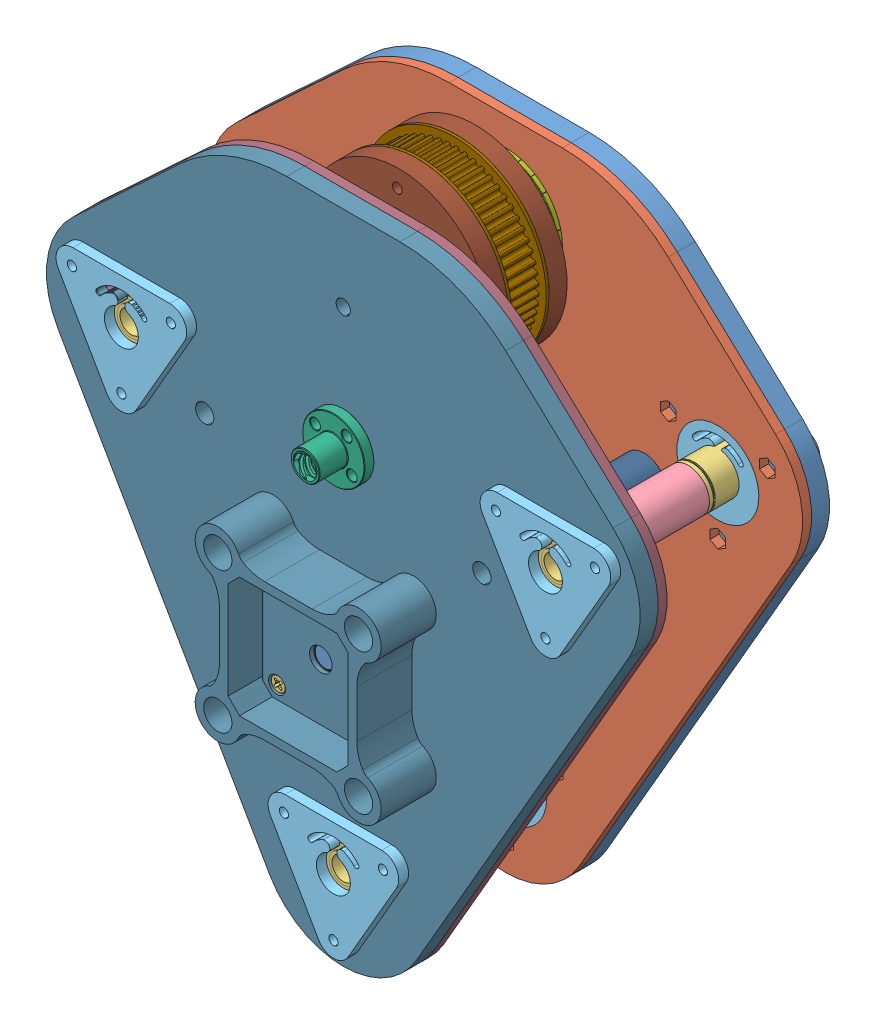
SolidWorks assembly assemblage_chariot, configuration Défaut. Lengths in mm.
Overall size (210 235.26 100).
51 component instances, 32 part files, 108 mates.
Components (placement in the parent):
- chariot_1_4_axe_z-1: chariot_1_4_axe_z [Défaut] at (104.2914 -77.7812 228.825) size (210 232 13.03)
- chariot_1_8_axe_z-1: chariot_1_8_axe_z [Défaut] at (104.2914 -77.7812 235.175) size (210 232 13.03)
- LM8UU-1: LM8UU [Default] at (179.2914 22.2188 238.825) x (-0.119175 0.992873 0) z (0 0 1) size (15 15 20)
- LM8UU-2: LM8UU [Default] at (104.2914 -107.7812 285.825) x (0.999936 0.011352 0) z (0 0 1) size (15 15 20)
- LM8UU-3: LM8UU [Default] at (29.2914 22.2188 285.825) x (0.609724 0.792614 0) z (0 0 1) size (15 15 20)
- LM8UU-4: LM8UU [Default] at (29.2914 22.2188 238.825) x (0.999283 -0.037866 0) z (0 0 1) size (15 15 20)
- LM8UU-5: LM8UU [Default] at (179.2914 22.2188 285.825) size (15 15 20)
- LM8UU-6: LM8UU [Default] at (104.2914 -107.7812 238.825) size (15 15 20)
- spacer_bearing_chariot-1: spacer_bearing_chariot [Défaut] at (104.2914 -107.7812 248.825) x (0.653682 -0.75677 0) z (0 0 1) size (15 15 27)
- spacer_bearing_chariot-2: spacer_bearing_chariot [Défaut] at (179.2914 22.2188 248.825) x (0.959506 -0.281688 0) z (0 0 1) size (15 15 27)
- spacer_bearing_chariot-3: spacer_bearing_chariot [Défaut] at (29.2914 22.2188 248.825) x (0.998603 0.052836 0) z (0 0 1) size (15 15 27)
- ancrage_bearing_lineaire-1: ancrage_bearing_lineaire [Défaut] at (179.2914 22.2188 299.325) x (-1 0 0) z (0 0 -1) size (46.22 41.63 13.03)
- ancrage_bearing_lineaire-2: ancrage_bearing_lineaire [Défaut] at (104.2914 -107.7812 299.325) x (-1 -0.000641 0) z (0 0 -1) size (46.22 41.63 13.03)
- ancrage_bearing_lineaire-3: ancrage_bearing_lineaire [Défaut] at (179.2914 22.2188 225.325) size (46.22 41.63 13.03)
- ancrage_bearing_lineaire-4: ancrage_bearing_lineaire [Défaut] at (104.2914 -107.7812 225.325) x (1 0.000641 0) z (0 0 1) size (46.22 41.63 13.03)
- ancrage_bearing_lineaire-5: ancrage_bearing_lineaire [Défaut] at (29.2914 22.2188 299.325) x (-1 -0.000641 0) z (0 0 -1) size (46.22 41.63 13.03)
- ancrage_bearing_lineaire-6: ancrage_bearing_lineaire [Défaut] at (29.2914 22.2188 225.325) size (46.22 41.63 13.03)
- Lead screw Nut tr8x8-4.step-1: Lead screw Nut tr8x8-4.step [Défaut] at (104.2914 22.2188 228.825) x (-0.445347 -0.895358 0) z (0 0 1) size (22 22 15)
- Lead screw Nut tr8x8-4.step-2: Lead screw Nut tr8x8-4.step [Défaut] at (104.2914 22.2188 295.825) x (0.811634 -0.584167 0) z (0 0 -1) size (22 22 15)
- 7806K755_Thrust Ball Bearing-1: 7806K755_Thrust Ball Bearing [7806K755] at (104.2914 64.2188 242.175) x (1 0 0) z (0 -1 0) size (40 14 40)
- 7806K755_Thrust Ball Bearing-2: 7806K755_Thrust Ball Bearing [7806K755] at (104.2914 64.2188 283.0983) x (-0.376178 0.926547 0) z (-0.926547 -0.376178 0) size (40 14 40)
- ThrustBallBearingUpper-1: ThrustBallBearingUpper [7806K755] at (104.2914 64.2188 242.1746) x (0.97097 0.239202 0) z (-0.239202 0.97097 0) size (40 14 40)
- ThrustBallBearingUpper-2: ThrustBallBearingUpper [7806K755] at (104.2914 64.2188 283.0986) x (0.933029 0.359801 0) z (0.359801 -0.933029 0) size (40 14 40)
- poulie_dente_modif-1: poulie_dente_modif [Výchozí] at (104.2914 64.2188 262.6366) x (0.023795 -0.999717 0) z (-0.999717 -0.023795 0) size (65 14.22 65)
- colonne_chariot-1: colonne_chariot [Défaut] at (153.3107 7.2188 238.35) size (16 16 48.51)
- colonne_chariot-2: colonne_chariot [Défaut] at (55.2722 7.2188 238.35) size (16 16 48.51)
- colonne_chariot-3: colonne_chariot [Défaut] at (104.2914 -79.7812 238.35) size (16 16 48.51)
- appuie_1_4_poulie-1: appuie_1_4_poulie [Default] at (104.2914 64.2188 255.5246) x (0.023795 -0.999717 0) z (0.999717 0.023795 0) size (65 6.35 65)
- appuie_1_4_poulie-2: appuie_1_4_poulie [Default] at (104.2914 64.2188 276.0986) x (-0.999717 -0.023795 0) z (0.023795 -0.999717 0) size (65 6.35 65)
- NEMA17 x 33.step-1: NEMA17 x 33.step [Défaut] at (104.2914 -39.7812 270.7486) x (1 0 0) z (0 -1 0) size (42 57 60)
  - Copper-2of4.step-1: Copper-2of4.step [Défaut] at (0 28 0) x (0 1 0) z (0 0 1) size (2.77 3.05 24)
  - Frontplate.step-1: Frontplate.step [Défaut] at (0 10.5 0) size (42 12.5 42)
  - Backplate.step-1: Backplate.step [Défaut] at (0 33 0) size (42 10.5 42)
  - Connenctor.step-1: Connenctor.step [Défaut] at (0 24.5 22) size (7 7 7)
  - Housing.step-1: Housing.step [Défaut] at (0 7.5 0) size (42 17 42)
  - Bearing dummy.step-1: Bearing dummy.step [Défaut] at (0 4 0) size (22 7 22)
  - Bearing dummy 01.step-1: Bearing dummy 01.step [Défaut] at (0 28 0) size (22 7 22)
  - Core.step-1: Core.step [Défaut] at origin size (30 55.5 30)
  - M3x25-Screw.step-1: M3x25-Screw.step [Défaut] at (15.5 30.6 15.5) x (1 0 0) z (0 1 0) size (5.5 5.5 27)
  - M3x25-Screw004.step-1: M3x25-Screw004.step [Défaut] at (-15.5 30.6 15.5) x (1 0 0) z (0 1 0) size (5.5 5.5 27)
  - M3x25-Screw005.step-1: M3x25-Screw005.step [Défaut] at (-15.5 30.6 -15.5) x (1 0 0) z (0 1 0) size (5.5 5.5 27)
  - M3x25-Screw006.step-1: M3x25-Screw006.step [Défaut] at (15.5 30.6 -15.5) x (1 0 0) z (0 1 0) size (5.5 5.5 27)
  - Cable-1of4.step-1: Cable-1of4.step [Défaut] at (0 28 0) size (3.44 3.69 21)
  - Copper-1of4.step-1: Copper-1of4.step [Défaut] at (0 28 0) size (2.77 3.05 24)
  - Cable-2of4.step-1: Cable-2of4.step [Défaut] at (0 28 0) x (0 1 0) z (0 0 1) size (3.44 3.69 21)
  - Copper-4of4.step-1: Copper-4of4.step [Défaut] at (0 28 0) x (0 -1 0) z (0 0 1) size (2.77 3.05 24)
  - Cable-3of4.step-1: Cable-3of4.step [Défaut] at (0 28 0) x (-1 0 0) z (0 0 1) size (3.44 3.69 21)
  - Copper-3of4.step-1: Copper-3of4.step [Défaut] at (0 28 0) x (-1 0 0) z (0 0 1) size (2.77 3.05 24)
  - Cable-4of4.step-1: Cable-4of4.step [Défaut] at (0 28 0) x (0 -1 0) z (0 0 1) size (3.44 3.69 21)
- chariot_1_8_axe_z_sans_trou_haut-2: chariot_1_8_axe_z_sans_trou_haut [Défaut] at (104.2914 -77.7812 286.3) size (210 232 13.03)
- chariot_1_4_axe_z_sans_trou_haut-2: chariot_1_4_axe_z_sans_trou_haut [Défaut] at (104.2914 -77.7812 289.475) size (210 232 29.35)
Mates (geometry in assembly coordinates):
- Coïncidente1: coincident anti-aligned: plane of chariot_1_4_axe_z-1 through (29.2914 22.2188 235.175) normal (0 0 1); plane of chariot_1_8_axe_z-1 through (29.2914 22.2188 235.175) normal (0 0 -1)
- Coaxiale1: concentric aligned: cylinder of chariot_1_4_axe_z-1 through (104.2914 22.2188 228.825) axis (0 0 1) radius 5.1; cylinder of chariot_1_8_axe_z-1 through (104.2914 22.2188 235.175) axis (0 0 1) radius 5.1
- Coaxiale2: concentric aligned: cylinder of chariot_1_4_axe_z-1 through (179.2914 22.2188 228.825) axis (0 0 1) radius 14.5; cylinder of chariot_1_8_axe_z-1 through (179.2914 22.2188 235.175) axis (0 0 1) radius 14.5
- Coïncidente2: coincident anti-aligned: plane of chariot_1_4_axe_z-2 through (29.2914 22.2188 290.007) normal (0 0 -1); plane of chariot_1_8_axe_z-2 through (29.2914 22.2188 290.007) normal (0 0 1)
- Coaxiale3: concentric aligned: cylinder of chariot_1_4_axe_z-2 through (179.2914 22.2188 290.007) axis (0 0 1) radius 14.5; cylinder of chariot_1_8_axe_z-2 through (179.2914 22.2188 286.832) axis (0 0 1) radius 8
- Coaxiale4: concentric aligned: cylinder of chariot_1_4_axe_z-2 through (104.2914 22.2188 290.007) axis (0 0 1) radius 5.1; cylinder of chariot_1_8_axe_z-2 through (104.2914 22.2188 286.832) axis (0 0 1) radius 5.1
- Coaxiale5: concentric aligned: cylinder of chariot_1_8_axe_z-1 through (29.2914 22.2188 235.175) axis (0 0 1) radius 14.5; cylinder of chariot_1_8_axe_z-2 through (29.2914 22.2188 286.832) axis (0 0 1) radius 8
- Coaxiale6: concentric aligned: cylinder of chariot_1_8_axe_z-1 through (179.2914 22.2188 235.175) axis (0 0 1) radius 14.5; cylinder of chariot_1_8_axe_z-2 through (179.2914 22.2188 286.832) axis (0 0 1) radius 8
- Coaxiale7: concentric anti-aligned: cylinder of chariot_1_8_axe_z-1 through (179.2914 22.2188 235.175) axis (0 0 1) radius 14.5; cylinder of LM8UU-1 through (179.2914 22.2188 248.825) axis (0 0 -1) radius 7.5
- Coaxiale8: concentric anti-aligned: cylinder of chariot_1_4_axe_z-1 through (104.2914 -107.7812 228.825) axis (0 0 1) radius 14.5; cylinder of LM8UU-6 through (104.2914 -107.7812 248.825) axis (0 0 -1) radius 7.5
- Coaxiale9: concentric anti-aligned: cylinder of chariot_1_4_axe_z-2 through (104.2914 -107.7812 290.007) axis (0 0 1) radius 14.5; cylinder of LM8UU-2 through (104.2914 -107.7812 295.825) axis (0 0 -1) radius 7.5
- Coaxiale10: concentric anti-aligned: cylinder of chariot_1_4_axe_z-2 through (29.2914 22.2188 290.007) axis (0 0 1) radius 14.5; cylinder of LM8UU-3 through (29.2914 22.2188 295.825) axis (0 0 -1) radius 7.5
- Coaxiale11: concentric anti-aligned: cylinder of chariot_1_4_axe_z-2 through (179.2914 22.2188 290.007) axis (0 0 1) radius 14.5; cylinder of LM8UU-5 through (179.2914 22.2188 295.825) axis (0 0 -1) radius 7.5
- Coaxiale12: concentric anti-aligned: cylinder of chariot_1_8_axe_z-1 through (29.2914 22.2188 235.175) axis (0 0 1) radius 14.5; cylinder of LM8UU-4 through (29.2914 22.2188 248.825) axis (0 0 -1) radius 7.5
- Coïncidente3: coincident aligned: plane of chariot_1_4_axe_z-1 through (29.2914 22.2188 228.825) normal (0 0 -1); plane of LM8UU-1 through (179.2914 22.2188 228.825) normal (0 0 -1)
- Coïncidente4: coincident aligned: plane of chariot_1_4_axe_z-1 through (29.2914 22.2188 228.825) normal (0 0 -1); plane of LM8UU-6 through (104.2914 -107.7812 228.825) normal (0 0 -1)
- Coïncidente5: coincident aligned: plane of chariot_1_4_axe_z-2 through (29.2914 22.2188 296.357) normal (0 0 1); plane of LM8UU-2 through (104.2914 -107.7812 295.825) normal (0 0 1)
- Coïncidente6: coincident aligned: plane of chariot_1_4_axe_z-2 through (29.2914 22.2188 296.357) normal (0 0 1); plane of LM8UU-5 through (179.2914 22.2188 295.825) normal (0 0 1)
- Coïncidente7: coincident aligned: plane of chariot_1_4_axe_z-2 through (29.2914 22.2188 296.357) normal (0 0 1); plane of LM8UU-3 through (29.2914 22.2188 295.825) normal (0 0 1)
- Coïncidente8: coincident aligned: plane of chariot_1_4_axe_z-1 through (29.2914 22.2188 228.825) normal (0 0 -1); plane of LM8UU-4 through (29.2914 22.2188 228.825) normal (0 0 -1)
- Distance1: distance = 48.482 mm anti-aligned: plane of chariot_1_8_axe_z-2 through (29.2914 22.2188 286.832) normal (0 0 -1); plane of chariot_1_8_axe_z-1 through (29.2914 22.2188 238.35) normal (0 0 1)
- Coaxiale13: concentric aligned: cylinder of LM8UU-1 through (179.2914 22.2188 248.825) axis (0 0 -1) radius 7.5; cylinder of spacer_bearing_chariot-2 through (179.2914 22.2188 275.825) axis (0 0 -1) radius 7.5
- Coïncidente10: coincident anti-aligned: plane of LM8UU-1 through (179.2914 22.2188 248.825) normal (0 0 1); plane of spacer_bearing_chariot-2 through (179.2914 22.2188 248.825) normal (0 0 -1)
- Coaxiale14: concentric aligned: cylinder of LM8UU-6 through (104.2914 -107.7812 248.825) axis (0 0 -1) radius 7.5; cylinder of spacer_bearing_chariot-1 through (104.2914 -107.7812 275.825) axis (0 0 -1) radius 7.5
- Coïncidente11: coincident anti-aligned: plane of LM8UU-6 through (104.2914 -107.7812 248.825) normal (0 0 1); plane of spacer_bearing_chariot-1 through (104.2914 -107.7812 248.825) normal (0 0 -1)
- Coaxiale16: concentric aligned: cylinder of LM8UU-4 through (29.2914 22.2188 248.825) axis (0 0 -1) radius 7.5; cylinder of spacer_bearing_chariot-3 through (29.2914 22.2188 275.825) axis (0 0 -1) radius 7.5
- Coïncidente12: coincident anti-aligned: plane of LM8UU-4 through (29.2914 22.2188 248.825) normal (0 0 1); plane of spacer_bearing_chariot-3 through (29.2914 22.2188 248.825) normal (0 0 -1)
- Coaxiale17: concentric anti-aligned: cylinder of chariot_1_4_axe_z-1 through (104.2914 -107.7812 228.825) axis (0 0 1) radius 14.5; cylinder of ancrage_bearing_lineaire-4 through (104.2914 -107.7812 238.35) axis (0 0 -1) radius 14.5
- Coïncidente13: coincident anti-aligned: circle of chariot_1_4_axe_z-1; cylinder of ancrage_bearing_lineaire-4 through (104.3044 -127.9885 228.825) axis (0 0 -1) radius 1.625
- Coaxiale18: concentric anti-aligned: cylinder of chariot_1_4_axe_z-1 through (86.7849 -97.6888 228.825) axis (0 0 1) radius 1.625; cylinder of ancrage_bearing_lineaire-4 through (86.7849 -97.6888 228.825) axis (0 0 -1) radius 1.625
- Coïncidente14: coincident anti-aligned: plane of chariot_1_4_axe_z-1 through (29.2914 22.2188 228.825) normal (0 0 -1); plane of ancrage_bearing_lineaire-4 through (104.2914 -107.7812 228.825) normal (0 0 1)
- Coïncidente15: coincident anti-aligned: plane of chariot_1_4_axe_z-1 through (29.2914 22.2188 228.825) normal (0 0 -1); plane of ancrage_bearing_lineaire-6 through (29.2914 22.2188 228.825) normal (0 0 1)
- Coaxiale19: concentric anti-aligned: cylinder of chariot_1_4_axe_z-1 through (29.2914 22.2188 228.825) axis (0 0 1) radius 14.5; cylinder of ancrage_bearing_lineaire-6 through (29.2914 22.2188 238.35) axis (0 0 -1) radius 7.5
- Coaxiale20: concentric anti-aligned: cylinder of chariot_1_4_axe_z-1 through (29.2914 2.0115 225.325) axis (0 0 1) radius 1.625; cylinder of ancrage_bearing_lineaire-6 through (29.2914 2.0115 228.825) axis (0 0 -1) radius 1.625
- Coaxiale21: concentric anti-aligned: cylinder of chariot_1_4_axe_z-1 through (11.7914 32.3224 225.325) axis (0 0 1) radius 1.625; cylinder of ancrage_bearing_lineaire-6 through (11.7914 32.3224 228.825) axis (0 0 -1) radius 1.625
- Coaxiale22: concentric anti-aligned: cylinder of chariot_1_4_axe_z-1 through (179.2914 22.2188 228.825) axis (0 0 1) radius 14.5; cylinder of ancrage_bearing_lineaire-3 through (179.2914 22.2188 238.35) axis (0 0 -1) radius 7.5
- Coaxiale23: concentric anti-aligned: cylinder of chariot_1_4_axe_z-1 through (196.7914 32.3224 228.825) axis (0 0 1) radius 1.625; cylinder of ancrage_bearing_lineaire-3 through (196.7914 32.3224 228.825) axis (0 0 -1) radius 1.625
- Coaxiale24: concentric anti-aligned: cylinder of chariot_1_4_axe_z-1 through (161.7914 32.3224 228.825) axis (0 0 1) radius 1.625; cylinder of ancrage_bearing_lineaire-3 through (161.7914 32.3224 228.825) axis (0 0 -1) radius 1.625
- Coïncidente16: coincident anti-aligned: plane of chariot_1_4_axe_z-1 through (29.2914 22.2188 228.825) normal (0 0 -1); plane of ancrage_bearing_lineaire-3 through (179.2914 22.2188 228.825) normal (0 0 1)
- Coaxiale25: concentric aligned: cylinder of chariot_1_4_axe_z-2 through (104.2914 -107.7812 290.007) axis (0 0 1) radius 14.5; cylinder of ancrage_bearing_lineaire-2 through (104.2914 -107.7812 286.3) axis (0 0 1) radius 7.5
- Coaxiale26: concentric aligned: cylinder of chariot_1_4_axe_z-2 through (86.7849 -97.6888 290.007) axis (0 0 1) radius 1.625; cylinder of ancrage_bearing_lineaire-2 through (86.7849 -97.6888 295.825) axis (0 0 1) radius 1.625
- Coïncidente17: coincident anti-aligned: plane of chariot_1_4_axe_z-2 through (29.2914 22.2188 296.357) normal (0 0 1); plane of ancrage_bearing_lineaire-2 through (104.2914 -107.7812 295.825) normal (0 0 -1)
- Coaxiale27: concentric aligned: cylinder of chariot_1_4_axe_z-2 through (179.2914 22.2188 290.007) axis (0 0 1) radius 14.5; cylinder of ancrage_bearing_lineaire-1 through (179.2914 22.2188 286.3) axis (0 0 1) radius 14.5
- Coaxiale28: concentric aligned: cylinder of chariot_1_4_axe_z-2 through (196.7914 32.3224 290.007) axis (0 0 1) radius 1.625; cylinder of ancrage_bearing_lineaire-1 through (196.7914 32.3224 295.825) axis (0 0 1) radius 1.625
- Coïncidente18: coincident anti-aligned: plane of chariot_1_4_axe_z-2 through (29.2914 22.2188 296.357) normal (0 0 1); plane of ancrage_bearing_lineaire-1 through (179.2914 22.2188 295.825) normal (0 0 -1)
- Coaxiale38: concentric aligned: cylinder of chariot_1_4_axe_z-2 through (46.7017 32.1893 290.007) axis (0 0 1) radius 1.625; cylinder of ancrage_bearing_lineaire-5 through (46.7849 32.3336 295.825) axis (0 0 1) radius 1.625
- Coaxiale41: concentric aligned: cylinder of chariot_1_4_axe_z-2 through (11.7017 32.1669 290.007) axis (0 0 1) radius 1.625; cylinder of ancrage_bearing_lineaire-5 through (11.7849 32.3112 295.825) axis (0 0 1) radius 1.625
- Coïncidente19: coincident anti-aligned: plane of chariot_1_4_axe_z-2 through (29.2914 22.2188 296.357) normal (0 0 1); plane of ancrage_bearing_lineaire-5 through (29.2914 22.2188 295.825) normal (0 0 -1)
- Coïncidente21: coincident anti-aligned: plane of chariot_1_4_axe_z-2 through (29.2914 22.2188 296.357) normal (0 0 1); plane of Lead screw Nut tr8x8-4.step-2 through (104.2914 22.2188 295.825) normal (0 0 -1)
- Coaxiale43: concentric anti-aligned: cylinder of chariot_1_4_axe_z-2 through (104.2914 22.2188 290.007) axis (0 0 1) radius 5.1; cylinder of Lead screw Nut tr8x8-4.step-2 through (104.2914 22.2188 309.325) axis (0 0 -1) radius 5.1
- Coaxiale44: concentric aligned: cylinder of chariot_1_4_axe_z-1 through (104.2914 22.2188 228.825) axis (0 0 1) radius 5.1; cylinder of Lead screw Nut tr8x8-4.step-1 through (104.2914 22.2188 215.325) axis (0 0 1) radius 5.1
- Coïncidente22: coincident anti-aligned: plane of chariot_1_4_axe_z-1 through (29.2914 22.2188 228.825) normal (0 0 -1); plane of Lead screw Nut tr8x8-4.step-1 through (104.2914 22.2188 228.825) normal (0 0 1)
- Coïncidente23: coincident anti-aligned: plane of chariot_1_4_axe_z-2 through (29.2914 22.2188 290.007) normal (0 0 -1); plane of 7806K755_Thrust Ball Bearing-2 through (108.1059 54.8236 290.0983) normal (0 0 1)
- Coaxiale45: concentric anti-aligned: cylinder of chariot_1_8_axe_z-2 through (104.2914 64.2188 286.832) axis (0 0 1) radius 20; cylinder of 7806K755_Thrust Ball Bearing-2 through (104.2914 64.2188 276.0983) axis (0 0 -1) radius 20
- Coïncidente24: coincident anti-aligned: plane of chariot_1_4_axe_z-1 through (29.2914 22.2188 235.175) normal (0 0 1); plane of 7806K755_Thrust Ball Bearing-1 through (94.1514 64.2188 235.175) normal (0 0 -1)
- Coaxiale46: concentric anti-aligned: cylinder of chariot_1_8_axe_z-1 through (104.2914 64.2188 235.175) axis (0 0 1) radius 20; cylinder of 7806K755_Thrust Ball Bearing-1 through (104.2914 64.2188 235.175) axis (0 0 -1) radius 20
- Parallèle1: parallel anti-aligned: plane of 7806K755_Thrust Ball Bearing-2 through (108.482 53.897 281.4045) normal (0 0 -1); plane of ThrustBallBearingUpper-2 through (85.7615 57.0731 280.8655) normal (0 0 1)
- Coaxiale48: concentric aligned: cylinder of 7806K755_Thrust Ball Bearing-2 through (104.2914 64.2188 290.0983) axis (0 0 1) radius 20; cylinder of ThrustBallBearingUpper-2 through (104.2914 64.2188 290.0986) axis (0 0 1) radius 20
- Distance2: distance = 0.539 mm anti-aligned: plane of ThrustBallBearingUpper-2 through (85.7615 57.0731 280.8655) normal (0 0 1); plane of 7806K755_Thrust Ball Bearing-2 through (108.482 53.897 281.4045) normal (0 0 -1)
- Parallèle2: parallel anti-aligned: plane of 7806K755_Thrust Ball Bearing-1 through (93.1514 64.2188 243.8688) normal (0 0 1); plane of ThrustBallBearingUpper-1 through (85.008 59.4682 244.4077) normal (0 0 -1)
- Coaxiale49: concentric aligned: cylinder of 7806K755_Thrust Ball Bearing-1 through (104.2914 64.2188 235.175) axis (0 0 -1) radius 20; cylinder of ThrustBallBearingUpper-1 through (104.2914 64.2188 235.1746) axis (0 0 -1) radius 20
- Distance3: distance = 0.539 mm anti-aligned: plane of 7806K755_Thrust Ball Bearing-1 through (93.1514 64.2188 243.8688) normal (0 0 1); plane of ThrustBallBearingUpper-1 through (85.008 59.4682 244.4077) normal (0 0 -1)
- Parallèle3: parallel anti-aligned: plane of ThrustBallBearingUpper-2 through (94.8305 60.5704 276.0986) normal (0 0 -1); plane of poulie_dente_modif-1 through (104.2914 64.2188 269.7486) normal (0 0 1)
- Coaxiale50: concentric anti-aligned: circle of chariot_1_8_axe_z-2; cylinder of poulie_dente_modif-1 through (104.2914 64.2188 253.6366) axis (0 0 -1) radius 32.5
- Coïncidente25: coincident anti-aligned: plane of chariot_1_8_axe_z-1 through (29.2914 22.2188 238.35) normal (0 0 1); plane of colonne_chariot-1 through (153.3107 7.2188 238.35) normal (0 0 -1)
- Coaxiale51: concentric aligned: cylinder of chariot_1_8_axe_z-2 through (153.3107 7.2188 296.357) axis (0 0 -1) radius 3.25; cylinder of colonne_chariot-1 through (153.3107 7.2188 286.864) axis (0 0 -1) radius 8
- Coïncidente26: coincident anti-aligned: plane of chariot_1_8_axe_z-1 through (29.2914 22.2188 238.35) normal (0 0 1); plane of colonne_chariot-3 through (104.2914 -79.7812 238.35) normal (0 0 -1)
- Coaxiale52: concentric aligned: cylinder of chariot_1_8_axe_z-2 through (104.2914 -79.7812 296.357) axis (0 0 -1) radius 3.25; cylinder of colonne_chariot-3 through (104.2914 -79.7812 286.864) axis (0 0 -1) radius 8
- Coaxiale53: concentric aligned: cylinder of chariot_1_8_axe_z-2 through (55.2722 7.2188 296.357) axis (0 0 -1) radius 3.25; cylinder of colonne_chariot-2 through (55.2722 7.2188 286.864) axis (0 0 -1) radius 8
- Coïncidente28: coincident anti-aligned: plane of chariot_1_8_axe_z-1 through (29.2914 22.2188 238.35) normal (0 0 1); plane of colonne_chariot-2 through (55.2722 7.2188 238.35) normal (0 0 -1)
- Coaxiale54: concentric anti-aligned: circle of ThrustBallBearingUpper-1; circle of appuie_1_4_poulie-1
- Coaxiale55: concentric aligned: circle of poulie_dente_modif-1; circle of appuie_1_4_poulie-1
- Coaxiale56: concentric anti-aligned: circle of poulie_dente_modif-1; cylinder of appuie_1_4_poulie-2 through (104.2914 64.2188 269.7486) axis (0 0 1) radius 32.5
- Coaxiale57: concentric aligned: circle of appuie_1_4_poulie-1; circle of appuie_1_4_poulie-2
- Coïncidente37: coincident anti-aligned: plane of poulie_dente_modif-1 through (104.2914 64.2188 269.7486) normal (0 0 1); plane of appuie_1_4_poulie-2 through (104.2914 64.2188 269.7486) normal (0 0 -1)
- Coïncidente39: coincident anti-aligned: plane of poulie_dente_modif-1 through (104.2914 64.2188 255.5246) normal (0 0 -1); plane of appuie_1_4_poulie-1 through (104.2914 64.2188 255.5246) normal (0 0 1)
- Distance4: distance = 0 mm anti-aligned: plane of ThrustBallBearingUpper-2 through (94.8305 60.5704 276.0986) normal (0 0 -1); plane of appuie_1_4_poulie-2 through (104.2914 64.2188 276.0986) normal (0 0 1)
- Coïncidente42: coincident aligned: plane of poulie_dente_modif-1 through (104.2914 64.2188 268.7486) normal (0 0 -1); plane of NEMA17 x 33.step-1/Frontplate.step-1 through (104.2914 -39.7812 268.7486) normal (0 0 -1)
- Coïncidente45: coincident anti-aligned: plane of NEMA17 x 33.step-1 through (104.2914 -39.7812 270.7486) normal (0 -1 0)
- Coïncidente46: coincident aligned: plane of chariot_1_4_axe_z-2 through (104.2914 -77.7812 290.007) normal (1 0 0); plane of NEMA17 x 33.step-1 through (104.2914 -39.7812 270.7486) normal (1 0 0)
- Coïncidente51: coincident anti-aligned: plane of ancrage_bearing_lineaire-5 through (29.2914 22.2188 295.825) normal (0 0 -1); plane of chariot_1_4_axe_z_sans_trou_haut-2 through (29.2914 22.2188 295.825) normal (0 0 1)
- Coaxiale63: concentric aligned: cylinder of ancrage_bearing_lineaire-5 through (29.2914 22.2188 286.3) axis (0 0 1) radius 14.5; cylinder of chariot_1_4_axe_z_sans_trou_haut-2 through (29.2914 22.2188 289.475) axis (0 0 1) radius 14.5
- Coaxiale65: concentric aligned: cylinder of chariot_1_4_axe_z-1 through (104.2914 64.2188 225.325) axis (0 0 1) radius 2.54; cylinder of chariot_1_4_axe_z_sans_trou_haut-2 through (104.2914 64.2188 285.975) axis (0 0 1) radius 2.54
- Coïncidente52: coincident anti-aligned: plane of ancrage_bearing_lineaire-1 through (179.2914 22.2188 295.825) normal (0 0 -1); plane of chariot_1_4_axe_z_sans_trou_haut-2 through (29.2914 22.2188 295.825) normal (0 0 1)
- Coïncidente53: coincident anti-aligned: plane of ancrage_bearing_lineaire-2 through (104.2914 -107.7812 295.825) normal (0 0 -1); plane of chariot_1_4_axe_z_sans_trou_haut-2 through (29.2914 22.2188 295.825) normal (0 0 1)
- Coaxiale66: concentric aligned: cylinder of ancrage_bearing_lineaire-2 through (104.2914 -107.7812 286.3) axis (0 0 1) radius 14.5; cylinder of chariot_1_4_axe_z_sans_trou_haut-2 through (104.2914 -107.7812 289.475) axis (0 0 1) radius 14.5
- Coaxiale67: concentric aligned: cylinder of ancrage_bearing_lineaire-2 through (104.3044 -127.9885 295.825) axis (0 0 1) radius 1.625; cylinder of chariot_1_4_axe_z_sans_trou_haut-2 through (104.3044 -127.9885 289.475) axis (0 0 1) radius 1.625
- Coaxiale68: concentric aligned: cylinder of ancrage_bearing_lineaire-1 through (179.2914 2.0115 295.825) axis (0 0 1) radius 1.625; cylinder of chariot_1_4_axe_z_sans_trou_haut-2 through (179.2914 2.0115 289.475) axis (0 0 1) radius 1.625
- Coaxiale69: concentric aligned: cylinder of ancrage_bearing_lineaire-1 through (179.2914 22.2188 286.3) axis (0 0 1) radius 14.5; cylinder of chariot_1_4_axe_z_sans_trou_haut-2 through (179.2914 22.2188 289.475) axis (0 0 1) radius 14.5
- Coïncidente54: coincident anti-aligned: plane of chariot_1_8_axe_z_sans_trou_haut-2 through (29.2914 22.2188 289.475) normal (0 0 1); plane of chariot_1_4_axe_z_sans_trou_haut-2 through (29.2914 22.2188 289.475) normal (0 0 -1)
- Coïncidente55: coincident aligned: plane of chariot_1_8_axe_z_sans_trou_haut-2 through (78.3059 -122.7729 289.475) normal (-0.866186 -0.499722 0); plane of chariot_1_4_axe_z_sans_trou_haut-2 through (78.3059 -122.7729 295.825) normal (-0.866186 -0.499722 0)
- Coïncidente56: coincident aligned: plane of chariot_1_8_axe_z_sans_trou_haut-2 through (46.8412 79.4988 289.475) normal (-0.680913 0.732365 0); plane of chariot_1_4_axe_z_sans_trou_haut-2 through (46.8412 79.4988 295.825) normal (-0.680913 0.732365 0)
- Coïncidente57: coincident anti-aligned: plane of Lead screw Nut tr8x8-4.step-2 through (104.2914 22.2188 295.825) normal (0 0 -1); plane of chariot_1_4_axe_z_sans_trou_haut-2 through (29.2914 22.2188 295.825) normal (0 0 1)
- Coïncidente60: coincident aligned: plane of chariot_1_4_axe_z-1 through (78.3059 -122.7729 235.175) normal (-0.866186 -0.499722 0); plane of chariot_1_4_axe_z_sans_trou_haut-2 through (78.3059 -122.7729 295.825) normal (-0.866186 -0.499722 0)
- Coaxiale70: concentric anti-aligned: cylinder of Lead screw Nut tr8x8-4.step-2 through (104.2914 22.2188 309.325) axis (0 0 -1) radius 5.1; cylinder of chariot_1_4_axe_z_sans_trou_haut-2 through (104.2914 22.2188 289.475) axis (0 0 1) radius 5.1
- Coïncidente61: coincident anti-aligned: plane of LM8UU-3 through (29.2914 22.2188 295.825) normal (0 0 1); plane of ancrage_bearing_lineaire-5 through (29.2914 22.2188 295.825) normal (0 0 -1)
- Coïncidente62: coincident anti-aligned: plane of LM8UU-3 through (29.2914 22.2188 275.825) normal (0 0 -1); plane of spacer_bearing_chariot-3 through (29.2914 22.2188 275.825) normal (0 0 1)
- Coaxiale71: concentric aligned: cylinder of LM8UU-3 through (29.2914 22.2188 295.825) axis (0 0 -1) radius 7.5; cylinder of spacer_bearing_chariot-3 through (29.2914 22.2188 275.825) axis (0 0 -1) radius 7.5
- Coïncidente63: coincident anti-aligned: plane of LM8UU-2 through (104.2914 -107.7812 295.825) normal (0 0 1); plane of ancrage_bearing_lineaire-2 through (104.2914 -107.7812 295.825) normal (0 0 -1)
- Coaxiale72: concentric aligned: cylinder of LM8UU-2 through (104.2914 -107.7812 295.825) axis (0 0 -1) radius 7.5; cylinder of spacer_bearing_chariot-1 through (104.2914 -107.7812 275.825) axis (0 0 -1) radius 7.5
- Coïncidente64: coincident anti-aligned: plane of LM8UU-5 through (179.2914 22.2188 295.825) normal (0 0 1); plane of ancrage_bearing_lineaire-1 through (179.2914 22.2188 295.825) normal (0 0 -1)
- Coaxiale73: concentric aligned: cylinder of LM8UU-5 through (179.2914 22.2188 295.825) axis (0 0 -1) radius 7.5; cylinder of spacer_bearing_chariot-2 through (179.2914 22.2188 275.825) axis (0 0 -1) radius 7.5
- Coïncidente65: coincident anti-aligned: plane of ThrustBallBearingUpper-1 through (94.4458 61.7933 249.1746) normal (0 0 1); plane of appuie_1_4_poulie-1 through (104.2914 64.2188 249.1746) normal (0 0 -1)
- Coaxiale74: concentric anti-aligned: cylinder of poulie_dente_modif-1 through (104.2914 64.2188 253.6366) axis (0 0 -1) radius 32.5; cylinder of appuie_1_4_poulie-1 through (104.2914 64.2188 249.1746) axis (0 0 1) radius 32.5
- Coïncidente66: coincident aligned: plane of chariot_1_4_axe_z-1 through (104.2914 -77.7812 228.825) normal (1 0 0); plane of NEMA17 x 33.step-1 through (104.2914 -39.7812 270.7486) normal (1 0 0)
- Coïncidente67: coincident anti-aligned: plane of NEMA17 x 33.step-1/Frontplate.step-1 through (104.2914 -39.7812 270.7486) normal (0 0 -1); plane of support_stepper_chariot-1 through (104.2914 -39.7812 270.7486) normal (0 0 1)
- Coïncidente68: coincident aligned: plane of NEMA17 x 33.step-1/Frontplate.step-1 through (121.262 -60.7812 281.2486) normal (0 -1 0); plane of support_stepper_chariot-1 through (87.3214 -60.7803 241.1746) normal (0 -1 0)
- Coaxiale75: concentric anti-aligned: circle of NEMA17 x 33.step-1/Frontplate.step-1; cylinder of support_stepper_chariot-1 through (88.7914 -24.2812 235.1746) axis (0 0 1) radius 1.5
